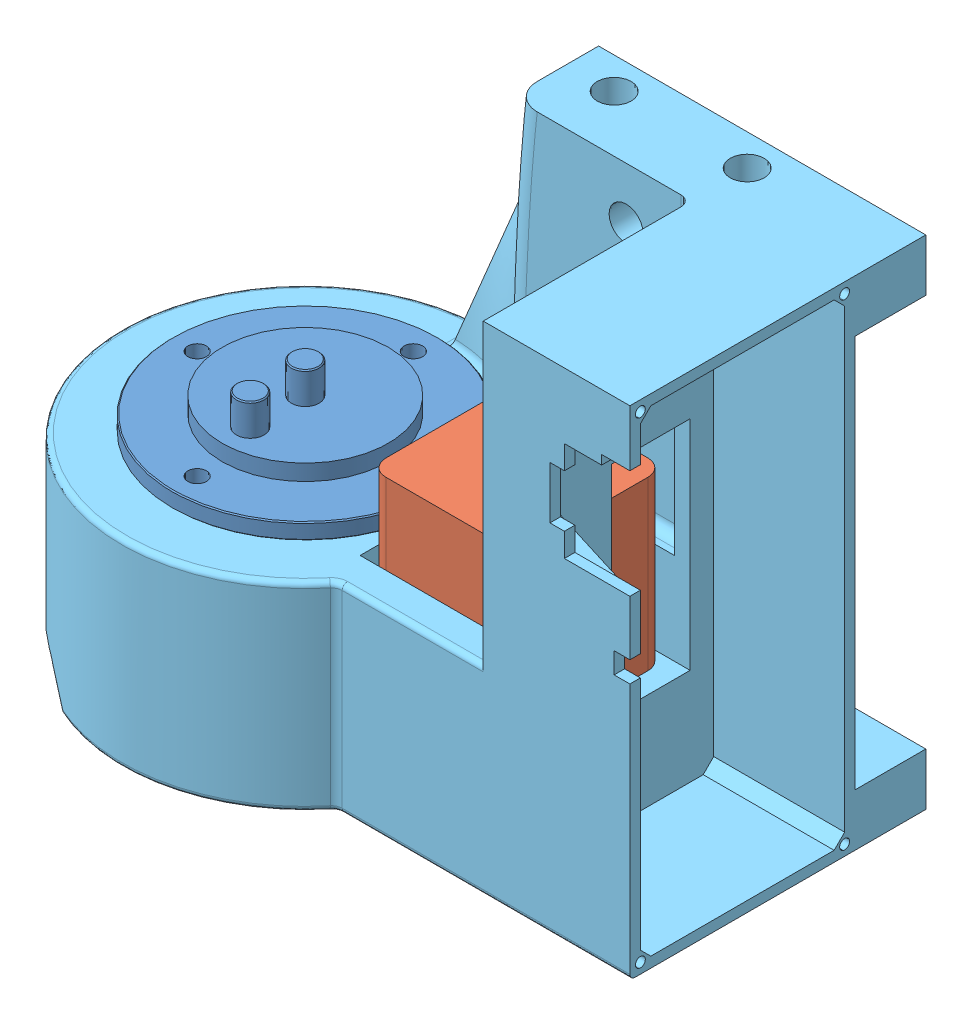
SolidWorks assembly dual_channel_commutator, configuration Default. Lengths in mm.
Overall size (118.5 107.25 70.26).
5 component instances, 5 part files, 0 mates.
Components (placement in the parent):
- BN_153127C0001_rotary_joint-1: BN_153127C0001_rotary_joint [Default] at origin size (50.8 55.9 50.8)
- 6627T370_POSITION-CONTROL DC MOTOR-1: 6627T370_POSITION-CONTROL DC MOTOR [6627T37] at (40.4432 -20.6733 0.0349) x (1 0 0) z (0 -1 0) size (28.19 28.19 52.07)
- gear_a-1: gear_a [Default] at (40.4581 -35.7604 0.0581) x (1 0 0) z (0 -1 0) size (21.12 21.05 5.08)
- gear_b_dual_channel-1: gear_b_dual_channel [Default] at (0.073 -35.9046 0.0567) x (1 0 0) z (0 -1 0) size (62.01 62.01 19.67)
- dual_channel_commutator_housing-1: dual_channel_commutator_housing [Default] at (-0.0093 -8.1808 0.0125) size (118.5 97.26 70.26)
